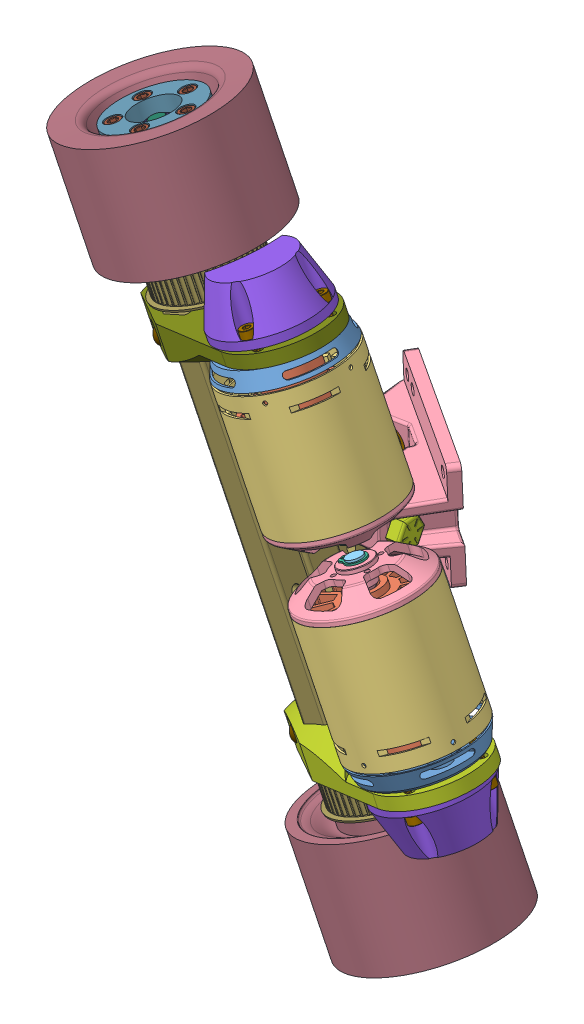
SolidWorks assembly MBS trucks pivot right, configuration Default. Lengths in mm.
Overall size (272.95 368.32 271.32).
89 component instances, 34 part files, 94 mates.
Components (placement in the parent):
- GPA26GT3150-A-N8-2: GPA26GT3150-A-N8 [Default] at (62.8793 -17.6552 -62.751) x (-0.357331 0.931448 0.068702) z (0.714319 0.319941 -0.622403) size (20 28 28)
  - GPA26GT3150-A-N8_b-1: GPA26GT3150-A-N8_b [Default] at origin size (20 28 28)
  - SET-SCREW4-3-1: SET-SCREW4-3 [Default] at (10 5.4 0) x (0 -1 0) z (-1 0 0) size (3 4 4)
  - SET-SCREW4-3-2: SET-SCREW4-3 [Default] at (10 -2.2723 -3.2919) x (0 0.568065 0.822984) z (-1 0 0) size (3 4 4)
- Key20mm-2: Key20mm [Default] at (65.3949 -16.7593 -61.8133) x (-0.714319 -0.319941 0.622403) z (-0.601717 -0.173328 -0.779676) size (3 20 3)
- MarkIITrucksCustomHanger pivor right-1: MarkIITrucksCustomHanger pivor right [Default] at (-31.1638 36.2817 -181.4556) x (-0.019038 0.999391 0.029249) z (0.838104 0 0.54551) size (362.13 183.87 195.64)
  - 50cal_baseplateEDIT-1: 50cal_baseplateEDIT [Default] at (40.8754 28.4427 48.4148) size (55.88 41.6 78.53)
  - BS_bushing-1: BS_bushing [Default] at (40.8754 74.2758 55.8381) x (0.903515 -0.328294 -0.275471) z (-0.428557 -0.692132 -0.580768) size (24.64 14.73 24.64)
  - BS_washer-1: BS_washer [Default] at (40.8754 63.8267 68.2909) x (0.781233 0.478195 0.401253) z (-0.624239 0.59846 0.502167) size (29.08 4.06 29.08)
  - kingpin-1: kingpin [Default] at (40.8754 51.905 82.4986) x (0.057682 0.764769 0.641717) z (0.998335 -0.044187 -0.037077) size (16.06 70.1 13.91)
  - kingpin-nut-1: kingpin-nut [90630A115] at (40.8754 87.1097 40.5433) x (0.976709 0.16437 0.137923) z (-0.214569 0.748202 0.627816) size (12.7 8.97 14.66)
  - Pivot_cup-1: Pivot_cup [Default] at (40.8754 44.9216 26.2393) x (-0.987309 0.102082 -0.121656) z (0.158811 0.63463 -0.756323) size (17.46 19.05 17.46)
  - RS_bushing-1: RS_bushing [Default] at (40.8754 76.7422 52.8988) x (0.999722 0.018072 0.015164) z (-0.023591 0.765831 0.642609) size (24.77 14.61 24.77)
  - washer-1: washer [Default] at (163.5053 116.6969 28.2009) x (-0.259291 0.957472 -0.126552) z (0.223038 0.186855 0.956734) size (11 1 11)
  - BS_washer-2: BS_washer [Default] at (40.8754 87.1097 40.5433) x (-0.947616 0.244683 0.205314) z (0.319411 0.725916 0.609116) size (29.08 4.06 29.08)
  - washer-2: washer [Default] at (187.2325 122.248 21.5854) x (0.339774 -0.687707 0.641571) z (-0.039134 -0.691901 -0.720931) size (11 1 11)
  - CustomHanger-1: CustomHanger [Default] at (40.8754 81.1126 56.6072) x (0.939693 0.219846 -0.262003) z (0.34202 -0.604023 0.719846) size (253 93.96 18)
  - KegelWheelAssembly-1: KegelWheelAssembly [Default] at (176.8088 165.9513 -23.4157) x (-0.321079 0.830973 -0.454305) z (0.11784 0.51103 0.851447) size (80 56 80)
    - Kegel 80mm longboard wheel-1: Kegel 80mm longboard wheel [Default] at (-60.1073 30.6906 17.2106) size (80 56 80)
    - 608-bearing-1: 608-bearing [6661K82] at (-60.1073 32.8534 17.2106) x (1 0 0) z (0 -1 0) size (22 22 7)
    - 608-bearing-2: 608-bearing [6661K82] at (-60.1073 15.6034 17.2106) x (-0.561464 0 0.827501) z (0 -1 0) size (22 22 7)
  - FPSSFJAD-D10-L64-T36-Q8-1: FPSSFJAD-D10-L64-T36-Q8 [Default] at (102.8951 102.5168 45.1001) x (0.939693 0.219846 -0.262003) z (0.305917 -0.197698 0.931306) size (100 10 10)
  - SetScrew_SAE_10-32x.5in-1: SetScrew_SAE_10-32x.5in [92313A829] at (125.4477 116.6557 46.2486) x (0.758718 0.418725 -0.499016) z (0 0.766044 0.642788) size (4.96 4.83 13.07)
  - SetScrew_SAE_10-32x.5in-3: SetScrew_SAE_10-32x.5in [92313A829] at (125.446 98.9319 31.3739) x (0.758718 0.418725 -0.499016) z (0 -0.766044 -0.642788) size (4.96 4.83 13.07)
  - NylonLockNut_5.16-24-1: NylonLockNut_5.16-24 [97135A225] at (187.7024 122.3579 21.4544) x (0.176745 0.34369 0.922301) z (-0.292812 0.912987 -0.284106) size (12.7 8.97 14.66)
  - KegelWheelAssembly-3: KegelWheelAssembly [Default] at (-133.6564 109.9576 93.5862) x (-0.321079 0.830973 -0.454305) z (-0.11784 -0.51103 -0.851447) size (80 56 80)
    - Kegel 80mm longboard wheel-1: Kegel 80mm longboard wheel [Default] at (-60.1073 30.6906 17.2106) size (80 56 80)
    - 608-bearing-1: 608-bearing [6661K82] at (-60.1073 32.8534 17.2106) x (1 0 0) z (0 -1 0) size (22 22 7)
    - 608-bearing-2: 608-bearing [6661K82] at (-60.1073 15.6034 17.2106) x (-0.561464 0 0.827501) z (0 -1 0) size (22 22 7)
  - FPSSFJAD-D10-L64-T36-Q8-3: FPSSFJAD-D10-L64-T36-Q8 [Default] at (-21.1443 73.4971 79.6845) x (-0.939693 -0.219846 0.262003) z (-0.305917 0.197698 -0.931306) size (100 10 10)
  - NylonLockNut_5.16-24-3: NylonLockNut_5.16-24 [97135A225] at (-105.9516 53.656 103.3302) x (-0.176745 -0.34369 -0.922301) z (-0.292812 0.912987 -0.284106) size (12.7 8.97 14.66)
  - SetScrew_SAE_10-32x.5in-7: SetScrew_SAE_10-32x.5in [92313A829] at (-43.6969 77.0851 93.407) x (-0.999936 0.007278 -0.008673) z (0 0.766044 0.642788) size (4.96 4.83 13.07)
  - SetScrew_SAE_10-32x.5in-8: SetScrew_SAE_10-32x.5in [92313A829] at (-43.6969 59.3582 78.536) x (-0.999936 0.007278 -0.008673) z (0 -0.766044 -0.642788) size (4.96 4.83 13.07)
- 91274A172_COATED ALLOY STEEL SOCKET HEAD CAP SCREW-1: 91274A172_COATED ALLOY STEEL SOCKET HEAD CAP SCREW [91274A172] at (17.1425 0.9134 -63.3166) x (0.185098 -0.198559 0.962452) z (0.926095 0.362892 -0.103239) size (9.53 9.53 32.48)
- 91274A172_COATED ALLOY STEEL SOCKET HEAD CAP SCREW-2: 91274A172_COATED ALLOY STEEL SOCKET HEAD CAP SCREW [91274A172] at (13.1465 1.7957 -96.0619) x (0.310502 -0.888509 -0.337846) z (0.926095 0.362892 -0.103239) size (9.53 9.53 32.48)
- 91274A172_COATED ALLOY STEEL SOCKET HEAD CAP SCREW-7: 91274A172_COATED ALLOY STEEL SOCKET HEAD CAP SCREW [91274A172] at (-42.5317 156.4652 -51.8433) x (-0.05291 -0.146013 -0.987867) z (0.926095 0.362892 -0.103239) size (9.53 9.53 32.48)
- Turnigy6374-6: Turnigy6374 [Default] at (42.3805 15.5078 -58.611) x (0.281637 0.177594 -0.942943) z (-0.890503 -0.317593 -0.32579) size (83.4 113.65 83.4)
  - Stator-1: Stator [Default] at (3.7873 1.8989 -6.3731) size (58.75 9.22 58.75)
  - StatorPart2-1: StatorPart2 [Default] at (3.7873 -16.3511 -6.3731) size (50 66 50)
  - AxelHoldCover-1: AxelHoldCover [Default] at (3.7873 -60.8511 -6.3731) x (0.982235 0 -0.187653) z (0.187653 0 0.982235) size (59.15 61.5 59.15)
  - AxelHold-1: AxelHold [Default] at (3.7873 -60.8511 -6.3731) x (0.729158 0 0.684345) z (0.684345 0 -0.729158) size (59 18.5 59)
  - AxisCust-1: AxisCust [Default] at (3.7873 -73.3511 -6.3731) x (0.844889 0 -0.534942) z (0.534942 0 0.844889) size (8 113.65 8)
  - 90967A120_STAINLESS STEEL EXTERNAL RETAINING RING-1: 90967A120_STAINLESS STEEL EXTERNAL RETAINING RING [90967A120] at (3.7873 12.2489 -6.3731) x (0 -1 0) z (0 0 1) size (0.8 12.1 9.85)
  - 90967A120_STAINLESS STEEL EXTERNAL RETAINING RING-2: 90967A120_STAINLESS STEEL EXTERNAL RETAINING RING [90967A120] at (3.7873 -73.7511 -6.3731) x (0 -1 0) z (-0.841191 0 -0.540738) size (0.8 12.1 9.85)
- MotorMountLeft-3: MotorMountLeft [Default] at (6.6736 -15.3581 -79.1058) x (-0.357331 0.931448 0.068702) z (-0.281637 -0.177594 0.942943) size (25.4 116.05 69.01)
- Belt Cap Wheel Side - Motor-2: Belt Cap Wheel Side - Motor [Default] at (55.3396 1.9983 -61.3013) x (-0.281637 -0.177594 0.942943) z (0.890503 0.317593 0.32579) size (50.8 25 40.64)
- M4x16mm_BlackZincSteel-3: M4x16mm_BlackZincSteel [91274A119] at (69.2858 20.879 -70.0775) x (0.925721 0.362972 -0.106266) z (-0.357331 0.931448 0.068702) size (7 7 20.35)
- M4x16mm_BlackZincSteel-4: M4x16mm_BlackZincSteel [91274A119] at (60.5233 15.3536 -40.7401) x (0.925721 0.362972 -0.106266) z (-0.357331 0.931448 0.068702) size (7 7 20.35)
- 92125A192_TYPE 18-8 SS FLAT-HEAD SOCKET CAP SCREW-9: 92125A192_TYPE 18-8 SS FLAT-HEAD SOCKET CAP SCREW [92125A192] at (45.7964 0.0068 -81.0244) x (-0.467555 -0.242075 0.850172) z (0.357331 -0.931448 -0.068702) size (8 8 12.4)
- 92125A192_TYPE 18-8 SS FLAT-HEAD SOCKET CAP SCREW-10: 92125A192_TYPE 18-8 SS FLAT-HEAD SOCKET CAP SCREW [92125A192] at (37.0339 -5.5187 -51.6869) x (0.925546 0.363007 -0.107656) z (0.357331 -0.931448 -0.068702) size (8 8 12.4)
- 91251A355_BLACK-OXIDE ALLOY STEEL SOCKET HEAD CAP SCREW-11: 91251A355_BLACK-OXIDE ALLOY STEEL SOCKET HEAD CAP SCREW [91251A355] at (10.6362 -18.0744 -95.0288) x (0.933519 0.353881 0.057548) z (-0.357331 0.931448 0.068702) size (7.92 7.92 68.91)
- GPA50GT3150-A-H26_b-1: GPA50GT3150-A-H26_b [Default] at (7.1203 -16.5224 -79.1916) x (0.357331 -0.931448 -0.068702) z (0.923966 0.341801 0.171633) size (20 51 51)
- Wheel Spacer 2-3: Wheel Spacer 2 [Default] at (21.2037 -53.2334 -81.8994) x (-0.155811 0.013078 -0.9877) z (0.92089 0.36364 -0.140457) size (44 14.02 44)
- Wheel Spacer Alum-3: Wheel Spacer Alum [Default] at (21.2037 -53.2334 -81.8994) x (-0.155811 0.013078 -0.9877) z (0.92089 0.36364 -0.140457) size (44 7.62 44)
- 91251A355_BLACK-OXIDE ALLOY STEEL SOCKET HEAD CAP SCREW-12: 91251A355_BLACK-OXIDE ALLOY STEEL SOCKET HEAD CAP SCREW [91251A355] at (-4.7856 -24.5937 -86.8527) x (0.31633 0.189908 -0.929446) z (-0.357331 0.931448 0.068702) size (7.92 7.92 68.91)
- 91251A355_BLACK-OXIDE ALLOY STEEL SOCKET HEAD CAP SCREW-13: 91251A355_BLACK-OXIDE ALLOY STEEL SOCKET HEAD CAP SCREW [91251A355] at (-1.8823 -24.8374 -68.4491) x (-0.738016 -0.236511 -0.631977) z (-0.357331 0.931448 0.068702) size (7.92 7.92 68.91)
- 91251A355_BLACK-OXIDE ALLOY STEEL SOCKET HEAD CAP SCREW-14: 91251A355_BLACK-OXIDE ALLOY STEEL SOCKET HEAD CAP SCREW [91251A355] at (15.3337 -18.4687 -65.2511) x (-0.772449 -0.33608 0.538863) z (-0.357331 0.931448 0.068702) size (7.92 7.92 68.91)
- 91251A355_BLACK-OXIDE ALLOY STEEL SOCKET HEAD CAP SCREW-15: 91251A355_BLACK-OXIDE ALLOY STEEL SOCKET HEAD CAP SCREW [91251A355] at (23.0706 -14.2889 -81.6783) x (0.260616 0.028802 0.965013) z (-0.357331 0.931448 0.068702) size (7.92 7.92 68.91)
- Wheel Spacer-3: Wheel Spacer [Default] at (21.2037 -53.2334 -81.8994) x (0.136385 0.124809 -0.982762) z (0.923966 0.341801 0.171633) size (44 7.02 44)
- 91274A172_COATED ALLOY STEEL SOCKET HEAD CAP SCREW-8: 91274A172_COATED ALLOY STEEL SOCKET HEAD CAP SCREW [91274A172] at (-42.5317 156.4652 -51.8433) x (-0.05291 -0.146013 -0.987867) z (0.926095 0.362892 -0.103239) size (9.53 9.53 32.48)
- 91274A172_COATED ALLOY STEEL SOCKET HEAD CAP SCREW-9: 91274A172_COATED ALLOY STEEL SOCKET HEAD CAP SCREW [91274A172] at (-46.5278 157.3474 -84.5886) x (0.376833 -0.903154 0.205696) z (0.926095 0.362892 -0.103239) size (9.53 9.53 32.48)
- Turnigy6374-7: Turnigy6374 [Default] at (-2.4422 165.9816 -43.6583) x (0.281637 0.177594 -0.942943) z (0.890503 0.317593 0.32579) size (83.4 113.65 83.4)
  - Stator-1: Stator [Default] at (3.7873 1.8989 -6.3731) size (58.75 9.22 58.75)
  - StatorPart2-1: StatorPart2 [Default] at (3.7873 -16.3511 -6.3731) size (50 66 50)
  - AxelHoldCover-1: AxelHoldCover [Default] at (3.7873 -60.8511 -6.3731) x (0.982235 0 -0.187653) z (0.187653 0 0.982235) size (59.15 61.5 59.15)
  - AxelHold-1: AxelHold [Default] at (3.7873 -60.8511 -6.3731) x (0.729158 0 0.684345) z (0.684345 0 -0.729158) size (59 18.5 59)
  - AxisCust-1: AxisCust [Default] at (3.7873 -73.3511 -6.3731) x (0.844889 0 -0.534942) z (0.534942 0 0.844889) size (8 113.65 8)
  - 90967A120_STAINLESS STEEL EXTERNAL RETAINING RING-1: 90967A120_STAINLESS STEEL EXTERNAL RETAINING RING [90967A120] at (3.7873 12.2489 -6.3731) x (0 -1 0) z (0 0 1) size (0.8 12.1 9.85)
  - 90967A120_STAINLESS STEEL EXTERNAL RETAINING RING-2: 90967A120_STAINLESS STEEL EXTERNAL RETAINING RING [90967A120] at (3.7873 -73.7511 -6.3731) x (0 -1 0) z (-0.841191 0 -0.540738) size (0.8 12.1 9.85)
- Belt Cap Wheel Side - Motor-3: Belt Cap Wheel Side - Motor [Default] at (-13.2679 180.8363 -48.1105) x (0.281637 0.177594 -0.942943) z (0.890503 0.317593 0.32579) size (50.8 25 40.64)
- M4x16mm_BlackZincSteel-5: M4x16mm_BlackZincSteel [91274A119] at (9.2543 177.3622 -58.5355) x (0.925721 0.362972 -0.106266) z (0.357331 -0.931448 -0.068702) size (7 7 20.35)
- M4x16mm_BlackZincSteel-6: M4x16mm_BlackZincSteel [91274A119] at (0.4918 171.8368 -29.198) x (0.925721 0.362972 -0.106266) z (0.357331 -0.931448 -0.068702) size (7 7 20.35)
- 92125A192_TYPE 18-8 SS FLAT-HEAD SOCKET CAP SCREW-11: 92125A192_TYPE 18-8 SS FLAT-HEAD SOCKET CAP SCREW [92125A192] at (-22.6682 178.4721 -67.8611) x (0.467555 0.242075 -0.850172) z (-0.357331 0.931448 0.068702) size (8 8 12.4)
- 92125A192_TYPE 18-8 SS FLAT-HEAD SOCKET CAP SCREW-12: 92125A192_TYPE 18-8 SS FLAT-HEAD SOCKET CAP SCREW [92125A192] at (-31.4307 172.9467 -38.5236) x (0.925546 0.363007 -0.107656) z (-0.357331 0.931448 0.068702) size (8 8 12.4)
- 91251A355_BLACK-OXIDE ALLOY STEEL SOCKET HEAD CAP SCREW-16: 91251A355_BLACK-OXIDE ALLOY STEEL SOCKET HEAD CAP SCREW [91251A355] at (-61.5731 170.1525 -81.1454) x (0.933519 0.353881 0.057548) z (0.357331 -0.931448 -0.068702) size (7.92 7.92 68.91)
- GPA50GT3150-A-H26_b-2: GPA50GT3150-A-H26_b [Default] at (-62.3806 164.6441 -65.829) x (-0.357331 0.931448 0.068702) z (-0.923966 -0.341801 -0.171633) size (20 51 51)
- Wheel Spacer 2-4: Wheel Spacer 2 [Default] at (-76.464 201.3551 -63.1213) x (0.155811 -0.013078 0.9877) z (0.92089 0.36364 -0.140457) size (44 14.02 44)
- Wheel Spacer Alum-4: Wheel Spacer Alum [Default] at (-76.464 201.3551 -63.1213) x (0.155811 -0.013078 0.9877) z (0.92089 0.36364 -0.140457) size (44 7.62 44)
- Wheel Spacer-4: Wheel Spacer [Default] at (-76.464 201.3551 -63.1213) x (0.136385 0.124809 -0.982762) z (-0.923966 -0.341801 -0.171633) size (44 7.02 44)
- GPA26GT3150-A-N8-3: GPA26GT3150-A-N8 [Default] at (-13.661 181.8609 -48.0349) x (-0.357331 0.931448 0.068702) z (0.714319 0.319941 -0.622403) size (20 28 28)
  - GPA26GT3150-A-N8_b-1: GPA26GT3150-A-N8_b [Default] at origin size (20 28 28)
  - SET-SCREW4-3-1: SET-SCREW4-3 [Default] at (10 5.4 0) x (0 -1 0) z (-1 0 0) size (3 4 4)
  - SET-SCREW4-3-2: SET-SCREW4-3 [Default] at (10 -2.2723 -3.2919) x (0 0.568065 0.822984) z (-1 0 0) size (3 4 4)
- Key20mm-3: Key20mm [Default] at (-16.4868 201.9057 -43.3842) x (-0.714319 -0.319941 0.622403) z (0.601717 0.173328 0.779676) size (3 20 3)
- MotorMountRight-2: MotorMountRight [Default] at (-61.9339 163.4798 -65.9149) x (-0.357331 0.931448 0.068702) z (-0.281637 -0.177594 0.942943) size (25.4 116.05 69.01)
- 91251A355_BLACK-OXIDE ALLOY STEEL SOCKET HEAD CAP SCREW-17: 91251A355_BLACK-OXIDE ALLOY STEEL SOCKET HEAD CAP SCREW [91251A355] at (-49.1387 173.938 -67.7949) x (-0.260616 -0.028802 -0.965013) z (0.357331 -0.931448 -0.068702) size (7.92 7.92 68.91)
- 91251A355_BLACK-OXIDE ALLOY STEEL SOCKET HEAD CAP SCREW-18: 91251A355_BLACK-OXIDE ALLOY STEEL SOCKET HEAD CAP SCREW [91251A355] at (-56.8757 169.7583 -51.3677) x (-0.772449 -0.33608 0.538863) z (0.357331 -0.931448 -0.068702) size (7.92 7.92 68.91)
- 91251A355_BLACK-OXIDE ALLOY STEEL SOCKET HEAD CAP SCREW-19: 91251A355_BLACK-OXIDE ALLOY STEEL SOCKET HEAD CAP SCREW [91251A355] at (-74.0917 163.3895 -54.5657) x (-0.738016 -0.236511 -0.631977) z (0.357331 -0.931448 -0.068702) size (7.92 7.92 68.91)
- 91251A355_BLACK-OXIDE ALLOY STEEL SOCKET HEAD CAP SCREW-20: 91251A355_BLACK-OXIDE ALLOY STEEL SOCKET HEAD CAP SCREW [91251A355] at (-76.9949 163.6332 -72.9694) x (-0.31633 -0.189908 0.929446) z (0.357331 -0.931448 -0.068702) size (7.92 7.92 68.91)
Mates (geometry in assembly coordinates):
- Concentric1: concentric anti-aligned: cylinder of ? through (0 89.5 0) axis (0 -1 0) radius 6; cylinder of ? through (0 92.55 0) axis (0 1 0) radius 6
- Concentric2: concentric anti-aligned: cylinder of ? through (0 -26.5 0) axis (0 1 0) radius 4; cylinder of GPA26GT3150-A-N8-2/GPA26GT3150-A-N8_b-1 through (0 -6.5 0) axis (0 -1 0) radius 4
- Coincident1: coincident aligned: plane of ? through (0 -26.5 0) normal (0 -1 0); plane of GPA26GT3150-A-N8-2/GPA26GT3150-A-N8_b-1 through (0 -26.5 0) normal (0 -1 0)
- Coincident7: coincident anti-aligned: line of ? through (-1.5 -26.5 -2.5) axis (0 0 -1); line of GPA26GT3150-A-N8-2/GPA26GT3150-A-N8_b-1 through (-1.5 -26.5 -5.4) axis (0 0 1)
- Coincident8: coincident aligned: plane of GPA26GT3150-A-N8-2/GPA26GT3150-A-N8_b-1 through (62.8793 -17.6552 -62.751) normal (0.357331 -0.931448 -0.068702); plane of Key20mm-2 through (65.3949 -16.7593 -61.8133) normal (0.357331 -0.931448 -0.068702)
- Coincident9: coincident anti-aligned: plane of ? through (1.5 -6.5 -2.5) normal (0 0 -1); plane of Key20mm-2 through (-1.5 -6.5 -2.5) normal (0 0 1)
- Coincident10: coincident anti-aligned: plane of GPA26GT3150-A-N8-2/GPA26GT3150-A-N8_b-1 through (60.0534 2.3896 -58.1003) normal (-0.714319 -0.319941 0.622403); plane of Key20mm-2 through (58.2482 1.8696 -60.4393) normal (0.714319 0.319941 -0.622403)
- Concentric5: concentric anti-aligned: cylinder of MarkIITrucksCustomHanger pivor right-1/CustomHanger-1 through (-77.4086 -5.45 -20.7444) axis (0 -1 0) radius 9; cylinder of ? through (-77.4086 -27.45 -20.7444) axis (0 1 0) radius 11
- Coincident15: coincident anti-aligned: plane of ? through (-77.2299 -26.5 -21.3999) normal (0 1 0); plane of ? through (-51.5162 -26.5 -25.2476) normal (0 -1 0)
- Coincident28: coincident anti-aligned: plane of MarkIITrucksCustomHanger pivor right-1/CustomHanger-1; plane of ? through (-34.0921 -14.7886 -63.0299) normal (-0.017088 0 -0.999854)
- Coincident37: coincident aligned: plane of ? through (-44.2534 59.243 -27.1128) normal (-0.40707 0 0.913397); plane of ? through (38.0802 32.893 9.5804) normal (-0.40707 0 0.913397)
- Coincident38: coincident anti-aligned: plane of ? through (-30.006 52.893 -59.0817) normal (0 -1 0); plane of ? through (52.3276 52.893 -22.3885) normal (0 1 0)
- Coincident40: coincident anti-aligned: plane of ? through (0 0 0) normal (0 -1 0); plane of ? through (-73.3266 0 -32.3363) normal (0 1 0)
- Concentric12: concentric aligned: cylinder of ? through (0 -26.5 0) axis (0 1 0) radius 4; cylinder of ? through (0 -6.35 0) axis (0 1 0) radius 6
- Coincident41: coincident anti-aligned: plane of ?; plane of ? through (-51.7284 -27.45 -24.8099) normal (0 -1 0)
- Concentric17: concentric aligned: cylinder of MarkIITrucksCustomHanger pivor right-1/CustomHanger-1 through (-34.2459 -20.2386 -72.0286) axis (0 -1 0) radius 9; cylinder of ? through (-34.2459 -22.2386 -72.0286) axis (0 -1 0) radius 10
- Coincident43: coincident anti-aligned: plane of ?; plane of ? through (-34.2459 -42.2386 -72.0286) normal (0 -1 0)
- Concentric18: concentric anti-aligned: cylinder of ? through (-93.4436 208.55 -19.2392) axis (0 -1 0) radius 2.54; cylinder of ? through (-93.4436 193.63 -19.2392) axis (0 1 0) radius 2.413
- Coincident45: coincident anti-aligned: plane of ? through (-93.4436 193.63 -19.2392) normal (0 -1 0); plane of ? through (-93.4436 193.63 -19.2392) normal (0 1 0)
- Concentric19: concentric: cylinder of ? through (-93.4436 208.55 -19.2392) axis (0 -1 0) radius 2.54; cylinder of ? through (-93.4436 193.63 -19.2392) axis (0 1 0) radius 2.413
- Coincident47: coincident anti-aligned: plane of ? through (-93.4436 193.63 -19.2392) normal (0 -1 0); plane of ? through (-93.4436 193.63 -19.2392) normal (0 1 0)
- Coincident48: coincident anti-aligned: plane of ?; plane of ? through (-43.0816 192.3928 -91.4524) normal (-0.019038 0.999391 0.029249)
- Concentric28: concentric anti-aligned: cylinder of ? through (-15.3407 192.0809 -62.7407) axis (-0.019038 0.999391 0.029249) radius 2.9; cylinder of ? through (-16.2508 239.8547 -61.3425) axis (0.019038 -0.999391 -0.029249) radius 2.413
- Coincident56: coincident anti-aligned: plane of GPA26GT3150-A-N8-2/GPA26GT3150-A-N8_b-1 through (57.9104 1.4298 -56.233) normal (-0.601717 -0.173328 -0.779676); plane of Key20mm-2 through (60.0534 2.3896 -58.1003) normal (0.601717 0.173328 0.779676)
- Coincident58: coincident aligned: plane of GPA26GT3150-A-N8-2/GPA26GT3150-A-N8_b-1; plane of ? through (-22.9313 -22.2386 -48.6196) normal (0 1 0)
- Concentric38: concentric aligned: cylinder of MarkIITrucksCustomHanger pivor right-1/CustomHanger-1 through (-41.8828 -7.7386 -55.3957) axis (0.999854 0 -0.017088) radius 2.3813; cylinder of ? through (-80.4696 -7.7386 -54.7362) axis (0.999854 0 -0.017088) radius 5
- Concentric40: concentric aligned: cylinder of ? through (-81.0335 -7.7386 -87.7314) axis (0.999854 0 -0.017088) radius 5; cylinder of 91274A172_COATED ALLOY STEEL SOCKET HEAD CAP SCREW-2 through (-52.2253 -7.7386 -88.2237) axis (0.999854 0 -0.017088) radius 4.7625
- Concentric41: concentric aligned: cylinder of ? through (-80.4696 -7.7386 -54.7362) axis (0.999854 0 -0.017088) radius 5; cylinder of 91274A172_COATED ALLOY STEEL SOCKET HEAD CAP SCREW-1 through (-51.6614 -7.7386 -55.2286) axis (0.999854 0 -0.017088) radius 4.7625
- Coincident61: coincident anti-aligned: plane of ? through (-45.3123 -7.7386 -55.3371) normal (-0.999854 0 0.017088); plane of 91274A172_COATED ALLOY STEEL SOCKET HEAD CAP SCREW-1 through (-45.3123 -7.7386 -55.3371) normal (0.999854 0 -0.017088)
- Coincident62: coincident anti-aligned: plane of ? through (-45.8762 -7.7386 -88.3322) normal (-0.999854 0 0.017088); plane of 91274A172_COATED ALLOY STEEL SOCKET HEAD CAP SCREW-2 through (-45.8762 -7.7386 -88.3322) normal (0.999854 0 -0.017088)
- Coincident65: coincident anti-aligned: plane of MarkIITrucksCustomHanger pivor right-1/CustomHanger-1; plane of ? through (-40.595 4.2614 -71.9201) normal (0.999854 0 -0.017088)
- Coincident68: coincident anti-aligned: plane of ? through (-34.2459 -14.7886 -72.0286) normal (0 1 0); plane of Turnigy6374-6/Stator-1 through (52.6547 -14.7886 -33.3) normal (0 -1 0)
- Concentric46: concentric anti-aligned: cylinder of GPA26GT3150-A-N8-2/GPA26GT3150-A-N8_b-1 through (55.7326 0.9737 -61.3769) axis (0.357331 -0.931448 -0.068702) radius 4; cylinder of Turnigy6374-6/AxisCust-1 through (62.5755 -16.8635 -62.6926) axis (-0.357331 0.931448 0.068702) radius 4
- Coincident70: coincident anti-aligned: plane of Key20mm-2 through (58.2482 1.8696 -60.4393) normal (0.714319 0.319941 -0.622403); plane of Turnigy6374-6/AxisCust-1 through (60.1136 2.407 -58.0223) normal (-0.714319 -0.319941 0.622403)
- Concentric55: concentric aligned: cylinder of 91274A172_COATED ALLOY STEEL SOCKET HEAD CAP SCREW-1 through (-51.6614 -7.7386 -55.2286) axis (0.999854 0 -0.017088) radius 4.7625; cylinder of ? through (-80.4696 -7.7386 -54.7362) axis (0.999854 0 -0.017088) radius 3.175
- Coincident75: coincident anti-aligned: plane of 91274A172_COATED ALLOY STEEL SOCKET HEAD CAP SCREW-1; plane of ? through (-45.3123 -7.7386 -55.3371) normal (-0.999854 0 0.017088)
- Coincident76: coincident anti-aligned: plane of MarkIITrucksCustomHanger pivor right-1/CustomHanger-1; plane of ? through (-40.595 4.2614 -71.9201) normal (0.999854 0 -0.017088)
- Coincident77: coincident anti-aligned: plane of MarkIITrucksCustomHanger pivor right-1/CustomHanger-1; plane of ? through (-34.0921 -14.7886 -63.0299) normal (-0.017088 0 -0.999854)
- Concentric56: concentric aligned: cylinder of 91274A172_COATED ALLOY STEEL SOCKET HEAD CAP SCREW-2 through (-54.3819 -7.7386 -88.1869) axis (0.999854 0 -0.017088) radius 4.7625; cylinder of ? through (-81.0335 -7.7386 -87.7314) axis (0.999854 0 -0.017088) radius 5
- Concentric57: concentric aligned: cylinder of MarkIITrucksCustomHanger pivor right-1/CustomHanger-1 through (-41.8828 -7.7386 -55.3957) axis (0.999854 0 -0.017088) radius 2.3813; cylinder of ? through (-80.4696 -7.7386 -54.7362) axis (0.999854 0 -0.017088) radius 5
- Concentric58: concentric aligned: cylinder of 91274A172_COATED ALLOY STEEL SOCKET HEAD CAP SCREW-7 through (-51.6614 159.2614 -55.2286) axis (0.999854 0 -0.017088) radius 4.7625; cylinder of ? through (-80.4696 159.2614 -54.7362) axis (0.999854 0 -0.017088) radius 5
- Coincident78: coincident anti-aligned: plane of 91274A172_COATED ALLOY STEEL SOCKET HEAD CAP SCREW-7; plane of ? through (-45.3123 159.2614 -55.3371) normal (-0.999854 0 0.017088)
- Concentric59: concentric aligned: cylinder of 91274A172_COATED ALLOY STEEL SOCKET HEAD CAP SCREW-8 through (-52.2253 159.2614 -88.2237) axis (0.999854 0 -0.017088) radius 4.7625; cylinder of ? through (-81.0335 159.2614 -87.7314) axis (0.999854 0 -0.017088) radius 5
- Coincident79: coincident anti-aligned: plane of MarkIITrucksCustomHanger pivor right-1/CustomHanger-1; plane of ? through (-43.2446 -0.6886 -71.8748) normal (0.999854 0 -0.017088)
- Concentric60: concentric anti-aligned: cylinder of 91274A172_COATED ALLOY STEEL SOCKET HEAD CAP SCREW-2 through (-52.2253 -7.7386 -88.2237) axis (0.999854 0 -0.017088) radius 4.7625; circle of ?
- Coincident80: coincident anti-aligned: plane of 91274A172_COATED ALLOY STEEL SOCKET HEAD CAP SCREW-2; plane of ? through (-45.8762 -7.7386 -88.3322) normal (-0.999854 0 0.017088)
- Concentric61: concentric aligned: cylinder of MarkIITrucksCustomHanger pivor right-1/CustomHanger-1 through (-7.1257 -6.148 -93.802) axis (0.926095 0.362892 -0.103239) radius 2.3813; cylinder of 91274A172_COATED ALLOY STEEL SOCKET HEAD CAP SCREW-2 through (-16.257 -9.7261 -92.784) axis (0.926095 0.362892 -0.103239) radius 4.7625
- Concentric62: concentric aligned: cylinder of MarkIITrucksCustomHanger pivor right-1/CustomHanger-1 through (-41.8828 -7.7386 -55.3957) axis (0.999854 0 -0.017088) radius 2.3813; cylinder of ? through (-80.4696 -7.7386 -54.7362) axis (0.999854 0 -0.017088) radius 3.175
- Concentric63: concentric: cylinder of 91274A172_COATED ALLOY STEEL SOCKET HEAD CAP SCREW-1 through (-51.6614 -7.7386 -55.2286) axis (0.999854 0 -0.017088) radius 4.7625; cylinder of ? through (-80.4696 -7.7386 -54.7362) axis (0.999854 0 -0.017088) radius 5
- Coincident81: coincident anti-aligned: plane of 91274A172_COATED ALLOY STEEL SOCKET HEAD CAP SCREW-1; plane of ? through (-45.3123 -7.7386 -55.3371) normal (-0.999854 0 0.017088)
- Coincident86: coincident aligned: plane of GPA26GT3150-A-N8-2/GPA26GT3150-A-N8_b-1 through (62.8793 -17.6552 -62.751) normal (0.357331 -0.931448 -0.068702); plane of Turnigy6374-6/AxisCust-1 through (62.8793 -17.6552 -62.751) normal (0.357331 -0.931448 -0.068702)
- Coincident87: coincident anti-aligned: plane of MarkIITrucksCustomHanger pivor right-1/CustomHanger-1; plane of ? through (-33.8358 147.2614 -48.0321) normal (-0.017088 0 -0.999854)
- Concentric72: concentric aligned: cylinder of MarkIITrucksCustomHanger pivor right-1/CustomHanger-1 through (-62.8039 148.5215 -49.5834) axis (0.926095 0.362892 -0.103239) radius 2.3813; cylinder of 91274A172_COATED ALLOY STEEL SOCKET HEAD CAP SCREW-7 through (-71.9352 144.9434 -48.5654) axis (0.926095 0.362892 -0.103239) radius 4.7625
- Concentric73: concentric aligned: cylinder of 91274A172_COATED ALLOY STEEL SOCKET HEAD CAP SCREW-1 through (-12.261 -10.6084 -60.0388) axis (0.926095 0.362892 -0.103239) radius 4.7625; cylinder of MotorMountLeft-3 through (-66.1302 -31.7171 -54.0335) axis (0.926095 0.362892 -0.103239) radius 5
- Concentric74: concentric aligned: cylinder of 91274A172_COATED ALLOY STEEL SOCKET HEAD CAP SCREW-2 through (-16.257 -9.7261 -92.784) axis (0.926095 0.362892 -0.103239) radius 4.7625; cylinder of MotorMountLeft-3 through (-70.1262 -30.8349 -86.7788) axis (0.926095 0.362892 -0.103239) radius 5
- Coincident99: coincident anti-aligned: plane of MarkIITrucksCustomHanger pivor right-1/CustomHanger-1 through (-83.5078 192.1236 -71.5804) normal (-0.926095 -0.362892 0.103239); plane of MotorMountLeft-3 through (-3.9303 -12.7095 -77.7403) normal (0.926095 0.362892 -0.103239)
- Coincident100: coincident anti-aligned: plane of 91274A172_COATED ALLOY STEEL SOCKET HEAD CAP SCREW-1 through (-6.3803 -8.304 -60.6943) normal (0.926095 0.362892 -0.103239); plane of MotorMountLeft-3 through (-6.3803 -8.304 -60.6943) normal (-0.926095 -0.362892 0.103239)
- Coincident101: coincident anti-aligned: plane of 91274A172_COATED ALLOY STEEL SOCKET HEAD CAP SCREW-2 through (-10.3763 -7.4218 -93.4396) normal (0.926095 0.362892 -0.103239); plane of MotorMountLeft-3 through (-10.3763 -7.4218 -93.4396) normal (-0.926095 -0.362892 0.103239)
- Coincident108: coincident anti-aligned: plane of Turnigy6374-6/Stator-1 through (53.0705 7.913 -60.8651) normal (0.357331 -0.931448 -0.068702); plane of MotorMountLeft-3 through (4.4045 -9.4434 -78.6695) normal (-0.357331 0.931448 0.068702)
- Concentric92: concentric aligned: cylinder of Belt Cap Wheel Side - Motor-2 through (82.8644 -14.516 -72.6882) axis (-0.357331 0.931448 0.068702) radius 4; cylinder of M4x16mm_BlackZincSteel-3 through (76.4324 2.2501 -71.4516) axis (-0.357331 0.931448 0.068702) radius 3.5
- Concentric93: concentric aligned: cylinder of Belt Cap Wheel Side - Motor-2 through (74.1019 -20.0414 -43.3507) axis (-0.357331 0.931448 0.068702) radius 4; cylinder of M4x16mm_BlackZincSteel-4 through (67.67 -3.2754 -42.1141) axis (-0.357331 0.931448 0.068702) radius 3.5
- Coincident121: coincident anti-aligned: plane of Belt Cap Wheel Side - Motor-2 through (75.0031 5.9759 -71.1768) normal (0.357331 -0.931448 -0.068702); plane of M4x16mm_BlackZincSteel-3 through (75.0031 5.9759 -71.1768) normal (-0.357331 0.931448 0.068702)
- Coincident122: coincident anti-aligned: plane of Belt Cap Wheel Side - Motor-2 through (66.2406 0.4504 -41.8393) normal (0.357331 -0.931448 -0.068702); plane of M4x16mm_BlackZincSteel-4 through (66.2406 0.4504 -41.8393) normal (-0.357331 0.931448 0.068702)
- Coincident123: coincident anti-aligned: plane of MotorMountLeft-3 through (6.6736 -15.3581 -79.1058) normal (0.357331 -0.931448 -0.068702); plane of Belt Cap Wheel Side - Motor-2 through (55.3396 1.9983 -61.3013) normal (-0.357331 0.931448 0.068702)
- Tangent4: tangent anti-aligned: plane of MotorMountLeft-3; cone of ? through (71.8505 -7.1277 -46.5804) axis (-0.019038 0.999391 0.029249)
- Tangent5: tangent anti-aligned: plane of MotorMountLeft-3; cone of ? through (89.6321 -19.6632 -21.2486) axis (-0.019038 0.999391 0.029249)
- Tangent9: tangent anti-aligned: plane of MotorMountLeft-3; cone of ? through (89.6321 -19.6632 -21.2486) axis (-0.019038 0.999391 0.029249)
- Tangent10: tangent: plane of MotorMountLeft-3; curve of ?
- Concentric105: concentric anti-aligned: cylinder of Turnigy6374-6/Stator-1 through (89.3833 -6.6015 -20.8663) axis (0.019038 -0.999391 -0.029249) radius 1.8559; circle of ?
- Concentric106: concentric anti-aligned: cylinder of Turnigy6374-6/Stator-1 through (71.8325 -6.1841 -46.5528) axis (0.019038 -0.999391 -0.029249) radius 1.8559; circle of ?
- Concentric107: concentric anti-aligned: cylinder of Turnigy6374-6/Stator-1 through (68.0103 24.204 -69.8323) axis (0.357331 -0.931448 -0.068702) radius 1.8559; circle of M4x16mm_BlackZincSteel-3
- Concentric108: concentric anti-aligned: cylinder of Turnigy6374-6/Stator-1 through (59.2478 18.6785 -40.4948) axis (0.357331 -0.931448 -0.068702) radius 1.8559; cylinder of M4x16mm_BlackZincSteel-4 through (67.67 -3.2754 -42.1141) axis (-0.357331 0.931448 0.068702) radius 3.5
- Tangent18: tangent anti-aligned: plane of MotorMountLeft-3 through (12.3222 -11.7962 -98.0177) normal (0.053524 -0.784211 0.618181); cone of 92125A192_TYPE 18-8 SS FLAT-HEAD SOCKET CAP SCREW-9 through (44.9745 2.1491 -80.8664) axis (-0.357331 0.931448 0.068702)
- Tangent19: tangent anti-aligned: plane of MotorMountLeft-3 through (0.8358 -16.1474 -62.3794) normal (0.451818 -0.533055 -0.715341); cone of 92125A192_TYPE 18-8 SS FLAT-HEAD SOCKET CAP SCREW-10 through (36.212 -3.3764 -51.5289) axis (-0.357331 0.931448 0.068702)
- Concentric109: concentric anti-aligned: cylinder of Turnigy6374-6/Stator-1 through (31.5418 8.7973 -50.631) axis (0.357331 -0.931448 -0.068702) radius 1.8559; circle of 92125A192_TYPE 18-8 SS FLAT-HEAD SOCKET CAP SCREW-10
- Concentric110: concentric anti-aligned: cylinder of Turnigy6374-6/Stator-1 through (40.3043 14.3228 -79.9685) axis (0.357331 -0.931448 -0.068702) radius 1.8559; circle of 92125A192_TYPE 18-8 SS FLAT-HEAD SOCKET CAP SCREW-9
- Coincident124: coincident aligned: cone of MotorMountLeft-3 through (36.212 -3.3764 -51.5289) axis (-0.357331 0.931448 0.068702); cone of 92125A192_TYPE 18-8 SS FLAT-HEAD SOCKET CAP SCREW-10 through (36.212 -3.3764 -51.5289) axis (-0.357331 0.931448 0.068702)
- Coincident140: coincident anti-aligned: plane of ? through (-15.0116 238.8514 -69.4308) normal (0.019038 -0.999391 -0.029249); plane of ? through (-15.0116 238.8514 -69.4308) normal (-0.019038 0.999391 0.029249)
- Concentric122: concentric aligned: cylinder of MotorMountLeft-3 through (74.8781 6.3019 -71.1527) axis (-0.357331 0.931448 0.068702) radius 2; cylinder of M4x16mm_BlackZincSteel-3 through (76.4324 2.2501 -71.4516) axis (-0.357331 0.931448 0.068702) radius 3.5
- Concentric128: concentric anti-aligned: cylinder of 91251A355_BLACK-OXIDE ALLOY STEEL SOCKET HEAD CAP SCREW-11 through (35.0512 -81.7165 -99.723) axis (-0.357331 0.931448 0.068702) radius 3.9624; cylinder of Wheel Spacer Alum-3 through (33.3267 -77.2213 -99.3914) axis (0.357331 -0.931448 -0.068702) radius 3.9688
- Coincident145: coincident anti-aligned: plane of 91251A355_BLACK-OXIDE ALLOY STEEL SOCKET HEAD CAP SCREW-11 through (33.3267 -77.2213 -99.3914) normal (-0.357331 0.931448 0.068702); plane of Wheel Spacer Alum-3 through (33.3267 -77.2213 -99.3914) normal (0.357331 -0.931448 -0.068702)
- Coincident146: coincident aligned: circle of MarkIITrucksCustomHanger pivor right-1/KegelWheelAssembly-3/Kegel 80mm longboard wheel-1; circle of Wheel Spacer-3
- Concentric129: concentric aligned: cylinder of MarkIITrucksCustomHanger pivor right-1/KegelWheelAssembly-3/Kegel 80mm longboard wheel-1 through (4.178 -40.6347 -69.6143) axis (0.357331 -0.931448 -0.068702) radius 2.9; cylinder of Wheel Spacer-3 through (17.3992 -75.0983 -72.1563) axis (0.357331 -0.931448 -0.068702) radius 2.54
- Coincident147: coincident anti-aligned: plane of Wheel Spacer Alum-3 through (30.2574 -76.8337 -83.6401) normal (-0.357331 0.931448 0.068702); plane of Wheel Spacer-3 through (30.2574 -76.8337 -83.6401) normal (0.357331 -0.931448 -0.068702)
- Concentric130: concentric aligned: circle of Wheel Spacer Alum-3; circle of Wheel Spacer-3
- Concentric131: concentric aligned: circle of Wheel Spacer Alum-3; circle of Wheel Spacer-3
- Concentric132: concentric aligned: cylinder of MarkIITrucksCustomHanger pivor right-1/KegelWheelAssembly-3/Kegel 80mm longboard wheel-1 through (14.5349 -35.85 -80.6172) axis (-0.357331 0.931448 0.068702) radius 40; cylinder of GPA50GT3150-A-H26_b-1 through (14.2669 -35.1514 -80.5657) axis (-0.357331 0.931448 0.068702) radius 13
- Coincident148: coincident aligned: circle of MarkIITrucksCustomHanger pivor right-1/KegelWheelAssembly-3/Kegel 80mm longboard wheel-1; circle of Wheel Spacer 2-3
- Coincident149: coincident anti-aligned: plane of GPA50GT3150-A-H26_b-1 through (17.131 -32.5304 -101.2037) normal (0.357331 -0.931448 -0.068702); plane of Wheel Spacer 2-3 through (14.2669 -35.1514 -80.5657) normal (-0.357331 0.931448 0.068702)
- Concentric133: concentric aligned: cylinder of Wheel Spacer 2-3 through (6.0094 -52.7328 -88.9282) axis (-0.357331 0.931448 0.068702) radius 2.54; cylinder of 91251A355_BLACK-OXIDE ALLOY STEEL SOCKET HEAD CAP SCREW-12 through (17.9049 -83.7406 -91.2154) axis (-0.357331 0.931448 0.068702) radius 2.413
- Concentric134: concentric aligned: cylinder of GPA50GT3150-A-H26_b-1 through (1.0068 -39.6925 -87.9664) axis (-0.357331 0.931448 0.068702) radius 2; cylinder of 91251A355_BLACK-OXIDE ALLOY STEEL SOCKET HEAD CAP SCREW-12 through (17.9049 -83.7406 -91.2154) axis (-0.357331 0.931448 0.068702) radius 2.413
- Coincident154: coincident aligned: plane of MarkIITrucksCustomHanger pivor right-1/CustomHanger-1 through (-68.9044 161.4161 -74.1899) normal (-0.357331 0.931448 0.068702); plane of MotorMountRight-2 through (-61.9339 163.4798 -65.9149) normal (-0.357331 0.931448 0.068702)
- Coincident155: coincident anti-aligned: plane of MarkIITrucksCustomHanger pivor right-1/CustomHanger-1 through (-66.8381 198.6557 -73.4387) normal (0.926095 0.362892 -0.103239); plane of MotorMountRight-2 through (-51.33 160.8312 -67.2803) normal (-0.926095 -0.362892 0.103239)
- Coincident156: coincident anti-aligned: plane of MarkIITrucksCustomHanger pivor right-1/CustomHanger-1 through (-30.6046 71.1148 -48.04) normal (0.121093 -0.026735 0.992281); plane of MotorMountRight-2 through (-49.9515 139.1794 -43.8452) normal (-0.121093 0.026735 -0.992281)
